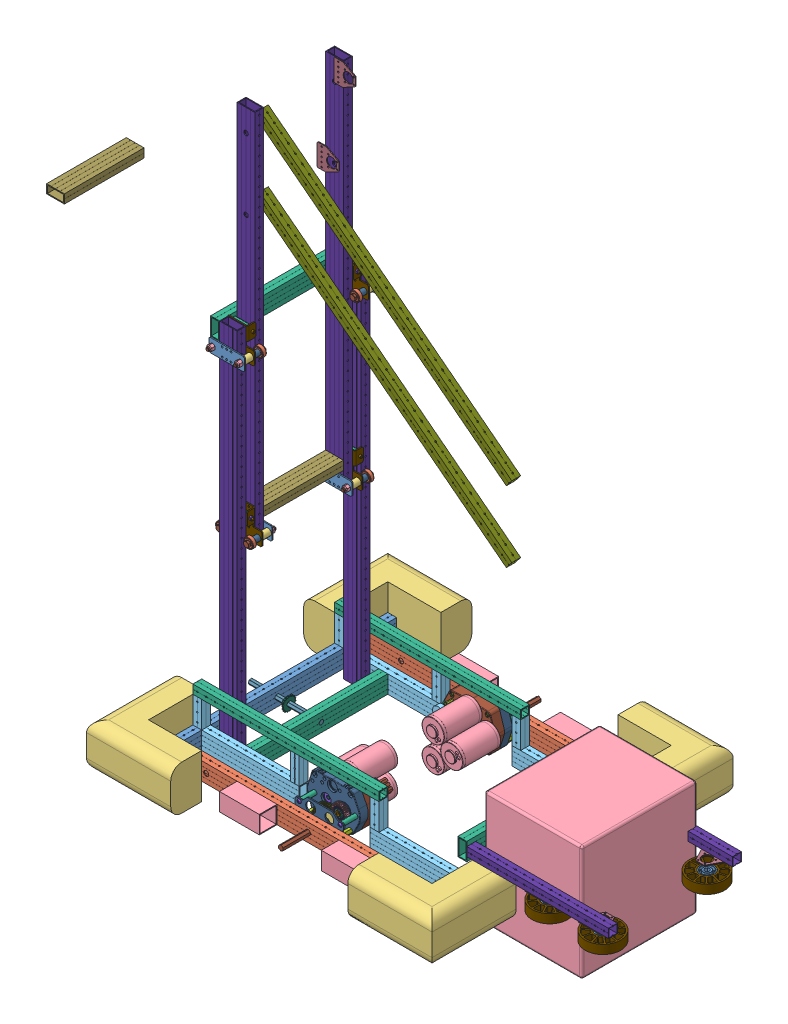
SolidWorks assembly Test Robot 1, configuration Default. Lengths in mm.
Overall size (1417.68 1634.47 868.53).
415 component instances, 100 part files, 60 mates.
Components (placement in the parent):
- Test Base 1-1: Test Base 1 [Default] at (-535.787 40.8668 506.935) size (990.6 169.11 863.6)
  - Base Rear Rail-1: Base Rear Rail [Default] at (282.1219 360.9185 104.1623) size (25.4 50.8 685.8)
  - Base Side Rail-1: Base Side Rail [Default] at (1044.1219 360.9185 789.9623) x (0 0 1) z (-1 0 0) size (25.4 50.8 762)
  - Base Side Rail-2: Base Side Rail [Default] at (1044.1219 360.9185 231.1623) x (0 0 1) z (-1 0 0) size (25.4 50.8 762)
  - Blue Bumper-1: Blue Bumper [Default] at (1171.1219 335.5185 942.3623) x (0 0 -1) z (1 0 0) size (241.3 127 241.3)
  - Blue Bumper-2: Blue Bumper [Default] at (1171.1219 335.5185 78.7623) x (-1 0 0) z (0 0 -1) size (241.3 127 241.3)
  - Bumper Support Bar-2: Bumper Support Bar [Default] at (879.0219 335.5185 166.0294) x (0 0 1) z (-1 0 0) size (50.8 50.8 114.3)
  - Bumper Support Bar-4: Bumper Support Bar [Default] at (586.9219 335.5185 166.0294) x (0 0 1) z (-1 0 0) size (50.8 50.8 114.3)
  - Bumper Support Bar-7: Bumper Support Bar [Default] at (586.9219 335.5185 801.0294) x (0 0 1) z (-1 0 0) size (50.8 50.8 114.3)
  - Bumper Support Bar-8: Bumper Support Bar [Default] at (879.0219 335.5185 801.0294) x (0 0 1) z (-1 0 0) size (50.8 50.8 114.3)
  - Base Side Rail Internal-1: Base Side Rail Internal [Default] at (307.5219 360.9185 307.3623) x (0 0 -1) z (1 0 0) size (25.4 50.8 279.4)
  - Base Side Rail Internal-2: Base Side Rail Internal [Default] at (307.5219 360.9185 713.7623) x (0 0 -1) z (1 0 0) size (25.4 50.8 279.4)
  - Base Side Rail Internal-3: Base Side Rail Internal [Default] at (1044.1219 360.9185 307.3623) x (0 0 1) z (-1 0 0) size (25.4 50.8 279.4)
  - Base Side Rail Internal-4: Base Side Rail Internal [Default] at (1044.1219 360.9185 713.7623) x (0 0 1) z (-1 0 0) size (25.4 50.8 279.4)
  - Frame Crossbar-1: Frame Crossbar [Default] at (1069.5219 360.9185 -48.2377) size (25.4 50.8 381)
  - Base Front Rail-1: Base Front Rail [Default] at (1069.5219 360.9185 104.1623) size (25.4 50.8 152.4)
  - 3 CIM Ball Shifter with WCD Output-1: 3 CIM Ball Shifter with WCD Output [Default] at (711.3612 400.7203 682.3171) x (0 1 0) z (0 0 1) size (169.11 183.68 312.65)
    - 217-2733-001 Rev2-1: 217-2733-001 Rev2 [Default] at (0 53.4162 37.6682) x (0 0 1) z (-0.00054 -1 0) size (7.11 24.61 24.61)
    - 217-2733-001 Rev2-2: 217-2733-001 Rev2 [Default] at (0 53.4162 7.9248) x (0 0 -1) z (-0.038475 0.99926 0) size (7.11 24.61 24.61)
    - 217-2731-001 Rev2-1: 217-2731-001 Rev2 [Default] at (0 0 0.0381) x (-0.099212 0.995066 0) z (0.995066 0.099212 0) size (31.12 7.94 31.12)
    - 217-2789-001 Rev2-1: 217-2789-001 Rev2 [Default] at (0 0 43.2943) x (0 0 -1) z (-0.58471 0.811243 0) size (11.1 38.4 38.4)
    - 217-2778-001 Rev2_NCQ8A075-050M_1-1: 217-2778-001 Rev2_NCQ8A075-050M_1 [Default] at (0 0 -53.848) x (-0.707107 0.707107 0) z (0 0 1) size (31.75 33.34 39.88)
      - 217-2778-002_075A-1: 217-2778-002_075A [Default] at origin size (31.75 33.34 26.92)
      - 217-2778-003_075M-1: 217-2778-003_075M [Default] at (0 0 -8.85) x (0.866025 -0.5 0) z (0 0 1) size (18.95 18.95 35.27)
      - 217-2778-004_075-1: 217-2778-004_075 [Default] at (0 0 10.362) size (21 20.74 0.97)
    - 217-2428-012 Rev2-1: 217-2428-012 Rev2 [Default] at (0 0 -40.386) size (63.5 22.23 2.29)
    - 217-2428-005 Rev1-1: 217-2428-005 Rev1 [Default] at (25.4 0 -19.05) x (-0.557362 -0.83027 0) z (-0.83027 0.557362 0) size (7.33 38.98 6.35)
    - 217-2428-005 Rev1-2: 217-2428-005 Rev1 [Default] at (-25.4 0 -19.05) x (0.667436 0.744667 0) z (0.744667 -0.667436 0) size (7.33 38.98 6.35)
    - SCREW-832-0375-1: SCREW-832-0375 [Default] at (25.4 0 -42.5958) x (0 0 1) z (-0.875404 0.483392 0) size (11.73 7.92 7.92)
    - SCREW-832-0375-2: SCREW-832-0375 [Default] at (-25.4 0 -42.5958) x (0 0 1) z (-0.966319 0.257347 0) size (11.73 7.92 7.92)
    - SCREW-832-0375-3: SCREW-832-0375 [Default] at (25.4 0 5.3848) x (0 0 -1) z (1 0 0) size (11.73 7.92 7.92)
    - SCREW-832-0375-4: SCREW-832-0375 [Default] at (-25.4 0 5.3848) x (0 0 -1) z (0.941463 -0.337115 0) size (11.73 7.92 7.92)
    - SBS1_SBS-0632-0250-1: SBS1_SBS-0632-0250 [Default] at (15.494 0 -36.2458) x (0 0 -1) z (0.854303 -0.519775 0) size (8.57 6.68 6.65)
    - SBS1_SBS-0632-0250-2: SBS1_SBS-0632-0250 [Default] at (-15.494 0 -36.2458) x (0 0 -1) z (0.854303 -0.519775 0) size (8.57 6.68 6.65)
    - 217-4098-100 Rev1-1: 217-4098-100 Rev1 [Default] at (0 0 -16.927) x (-0.503316 0.864103 0) z (0 0 1) size (18.03 19.79 22.46)
      - 217-4098-006 Rev2-1: 217-4098-006 Rev2 [Default] at (0 0 -4.6312) x (0 -1 0) z (0 0 -1) size (18.09 11.02 22.46)
      - 217-4098-006 Rev2-2: 217-4098-006 Rev2 [Default] at (0 0 -4.6312) x (0 1 0) z (0 0 -1) size (18.09 11.02 22.46)
      - 217-3489-001 Rev1-1: 217-3489-001 Rev1 [Default] at (0 0 -4.6312) x (0 0 1) z (-0.980217 -0.197926 0) size (4.77 12.7 12.7)
      - 97633A130_97633A130_grv-1: 97633A130_97633A130_grv [Default] at (0 0 -7.33) x (0 0 -1) z (0.979861 0.199683 0) size (0.64 8.74 7.34)
      - 91251A107_91251A107-1: 91251A107_91251A107 [Default] at (-4.8375 -6.735 -9.4343) x (0 0.863883 -0.503692) z (-1 0 0) size (4.65 4.65 10.79)
      - 91251A107_91251A107-2: 91251A107_91251A107 [Default] at (4.8375 6.735 -9.4343) x (0 0.470889 -0.882193) z (1 0 0) size (4.65 4.65 10.79)
    - 217-2428-017 Rev2-1: 217-2428-017 Rev2 [Default] at (12.7 -21.997 -3.614) x (-0.578458 -0.815712 0) z (0 0 -1) size (14.73 14.73 7.37)
    - 217-2428-016 Rev3_Spur01-1: 217-2428-016 Rev3_Spur01 [Default] at (0 0 -3.614) x (0.873157 -0.48744 0) z (0 0 1) size (40.67 40.74 13.32)
    - 217-2428-019 Rev1-1: 217-2428-019 Rev1 [Default] at (12.7 -21.997 -20.6248) x (0.866025 0.5 0) z (0 0 1) size (50.8 19.05 1.57)
    - 217-2428-006 Rev1-1: 217-2428-006 Rev1 [Default] at (32.079 -14.2875 -9.525) x (-0.752416 0.658689 0) z (0.658689 0.752416 0) size (7.33 19.93 6.35)
    - 217-2428-006 Rev1-2: 217-2428-006 Rev1 [Default] at (-3.6662 -34.925 -9.525) x (0.84498 0.534798 0) z (0.534798 -0.84498 0) size (7.33 19.93 6.35)
    - SCREW-832-0375-5: SCREW-832-0375 [Default] at (32.079 -14.2875 4.7498) x (0 0 -1) z (0.980613 0.195955 0) size (11.73 7.92 7.92)
    - SCREW-832-0375-6: SCREW-832-0375 [Default] at (-3.6662 -34.925 5.3848) x (0 0 -1) z (-0.672515 -0.740083 0) size (11.73 7.92 7.92)
    - SCREW-832-0375-7: SCREW-832-0375 [Default] at (-3.6662 -34.925 -22.8346) x (0 0 1) z (0.948865 0.315681 0) size (11.73 7.92 7.92)
    - SCREW-832-0375-8: SCREW-832-0375 [Default] at (32.079 -14.2875 -22.8346) x (0 0 1) z (-0.875404 0.483392 0) size (11.73 7.92 7.92)
    - 217-2614-001_12t-1: 217-2614-001_12t [Default] at (36.9798 39.6868 15.8623) x (-0.087156 0.996195 0) z (0 0 1) size (18.29 18.29 19)
    - 217-2761-001 rev1-1: 217-2761-001 rev1 [Default] at (33.1943 39.3556 16.1) x (0.087156 -0.996195 0) z (0 0 1) size (2 2 20)
    - 217-2761-001 rev1-2: 217-2761-001 rev1 [Default] at (-40.7653 40.018 16.1) x (0.087156 0.996195 0) z (0 0 1) size (2 2 20)
    - 217-2614-001_12t-2: 217-2614-001_12t [Default] at (-36.9798 39.6868 15.8623) x (0.087156 0.996195 0) z (0 0 1) size (18.29 18.29 19)
    - 217-2614-001_12t-3: 217-2614-001_12t [Default] at (0 92.8624 15.8623) x (0.97459 0.223996 0) z (0 0 1) size (18.29 18.29 19)
    - 217-2761-001 rev1-3: 217-2761-001 rev1 [Default] at (-0.8512 96.5658 16.1) x (0.97459 0.223996 0) z (0 0 1) size (2 2 20)
    - 217-3195-002 rev2-1: 217-3195-002 rev2 [Default] at (0 0 50.546) x (-1 0 0) z (0 0 -1) size (114.31 152.24 24.96)
    - 217-3195-001 Rev1-1: 217-3195-001 Rev1 [Default] at origin size (113.41 152.24 26.86)
    - Nylock Nut_NNY2520-ZC-1: Nylock Nut_NNY2520-ZC [Default] at (48.8823 73.025 37.846) x (0 0.866025 -0.5) z (-1 0 0) size (12.85 11.89 7.62)
    - Nylock Nut_NNY2520-ZC-2: Nylock Nut_NNY2520-ZC [Default] at (48.8823 -3.175 37.846) x (0 0 -1) z (-1 0 0) size (12.85 11.89 7.62)
    - Nylock Nut_NNY2520-ZC-3: Nylock Nut_NNY2520-ZC [Default] at (44.45 85.725 7.8613) x (0 1 0) z (0 0 -1) size (12.85 11.89 7.62)
    - 276-1027-001-1: 276-1027-001 [Default] at (47.625 58.1787 6.35) x (0 1 0) z (-1 0 0) size (8.61 5.64 9.94)
    - 276-1027-001-2: 276-1027-001 [Default] at (-47.625 58.1787 6.35) x (0 -1 0) z (1 0 0) size (8.61 5.64 9.94)
    - SCREW-832-1750-1: SCREW-832-1750 [Default] at (-47.625 58.1787 47.0408) x (0 0 -1) z (-0.960822 -0.277167 0) size (46.66 7.92 7.92)
    - SCREW-832-1750-2: SCREW-832-1750 [Default] at (47.625 58.1787 47.0408) x (0 0 -1) z (-0.960822 -0.277167 0) size (46.66 7.92 7.92)
    - Nylock Nut_NNY2520-ZC-4: Nylock Nut_NNY2520-ZC [Default] at (44.45 -15.875 7.8613) x (0 1 0) z (0 0 -1) size (12.85 11.89 7.62)
    - 217-2428-004 Rev3-1: 217-2428-004 Rev3 [Default] at (0 53.4162 22.7711) x (-0.709585 0.70462 0) z (0 0 1) size (11 9.53 43.92)
    - SBS1_SBS-2520-1625SS-1: SBS1_SBS-2520-1625SS [Default] at (44.45 85.725 42.4688) x (0 0 -1) z (-0.251219 0.96793 0) size (45.3 11.2 11.18)
    - SBS1_SBS-2520-1625SS-2: SBS1_SBS-2520-1625SS [Default] at (44.45 -15.875 42.4688) x (0 0 -1) z (-0.251219 0.96793 0) size (45.3 11.2 11.18)
    - SBS1_SBS2520-1750-1: SBS1_SBS2520-1750 [Default] at (-44.45 85.725 7.4422) x (0 0 1) z (-0.031478 0.999504 0) size (48.48 11.22 11.17)
    - SBS1_SBS2520-1750-2: SBS1_SBS2520-1750 [Default] at (-44.45 -15.875 7.4422) x (0 0 1) z (-0.937114 -0.349025 0) size (48.48 11.22 11.17)
    - 217-2428-021 Rev1-1: 217-2428-021 Rev1 [Default] at (0 53.4162 9.5123) x (0.451333 -0.892356 0) z (0 0 1) size (15.88 15.88 3.17)
    - 217-2428-029 Rev1-1: 217-2428-029 Rev1 [Default] at (0 53.4162 36.957) x (0.999846 0.017557 0) z (0 0 1) size (15.88 15.88 1.12)
    - Grayhill Lock Washer-1: Grayhill Lock Washer [Default] at (12.7 -21.997 -18.6817) x (0.467173 -0.884166 0) z (0 0 1) size (19.69 19.69 0.74)
    - Grayhill Nut-1: Grayhill Nut [Default] at (12.7 -21.997 -17.0434) x (0.984088 0.177684 0) z (0 0 1) size (18.33 15.88 2.54)
    - 217-2000-1: 217-2000 [Default] at (0 92.8624 0) x (0 0 -1) z (0.223996 -0.97459 0) size (150.2 64.01 64.01)
    - 217-2000-2: 217-2000 [Default] at (-36.9798 39.6868 0) x (0 0 -1) z (0.996195 -0.087156 0) size (150.2 64.01 64.01)
    - 217-2000-3: 217-2000 [Default] at (36.9798 39.6868 0) x (0 0 -1) z (0.996195 0.087156 0) size (150.2 64.01 64.01)
    - Grahill Encoder-1: Grahill Encoder [Default] at (12.7 -21.997 -16.1798) x (-0.580071 0.814566 0) z (-0.814566 -0.580071 0) size (31.75 31.12 31.75)
    - 217-3195-009 Rev1_wcd 2-1: 217-3195-009 Rev1_wcd 2 [Default] at (0 85.725 50.546) x (-0.998427 -0.056065 0) z (0 0 1) size (12.7 12.7 41.27)
    - 217-3195-006 Rev1_WCD-1: 217-3195-006 Rev1_WCD [Default] at (-44.45 85.725 44.1452) x (0.5 0.866025 0) z (0 0 1) size (12.7 14.66 47.62)
    - 217-3195-009 Rev1_wcd 2-2: 217-3195-009 Rev1_wcd 2 [Default] at (0 -31.75 50.546) x (0.947633 0.319361 0) z (0 0 1) size (12.7 12.7 41.27)
    - 217-3195-006 Rev1_WCD-2: 217-3195-006 Rev1_WCD [Default] at (-44.45 -15.875 44.1452) x (0.5 -0.866025 0) z (0 0 1) size (12.7 14.66 47.62)
    - Nylock Nut_NNY2520-ZC-5: Nylock Nut_NNY2520-ZC [Default] at (0 -31.75 45.0723) x (-0.5 0.866025 0) z (0 0 -1) size (12.85 11.89 7.62)
    - Nylock Nut_NNY2520-ZC-6: Nylock Nut_NNY2520-ZC [Default] at (0 85.725 45.0723) x (-0.5 0.866025 0) z (0 0 -1) size (12.85 11.89 7.62)
    - SBS1_SBS-2520-2250-1: SBS1_SBS-2520-2250 [Default] at (0 -31.75 98.298) x (0 0 -1) z (-0.933488 -0.358607 0) size (61.18 11.22 11.17)
    - SBS1_SBS2520-0625ZC-1: SBS1_SBS2520-0625ZC [Default] at (-44.45 85.725 98.298) x (0 0 -1) z (0.400817 0.916158 0) size (19.57 11.22 11.17)
    - SBS1_SBS2520-0625ZC-2: SBS1_SBS2520-0625ZC [Default] at (-44.45 -15.875 98.298) x (0 0 -1) z (-0.75178 -0.659414 0) size (19.57 11.22 11.17)
    - SBS1_SBS-2520-2250-2: SBS1_SBS-2520-2250 [Default] at (0 85.725 98.298) x (0 0 -1) z (0.056677 -0.998393 0) size (61.18 11.22 11.17)
    - 217-3195-003 rev2-1: 217-3195-003 rev2 [Default] at (0 0 94.9452) size (88.62 139.7 3.17)
    - 217-2617-003 Rev1-1: 217-2617-003 Rev1 [Default] at (-39.878 35.5392 121.8535) x (-0.5 -0.866025 0) z (0 0 1) size (14.66 12.7 152.4)
    - 217-3109-001 Rev1-1: 217-3109-001 Rev1 [Default] at (-39.878 35.5392 49.1808) x (0 0 1) z (0.312889 -0.94979 0) size (7.94 28.57 28.57)
    - 217-2734-001 Rev3-1: 217-2734-001 Rev3 [Default] at (-39.878 35.5392 98.1202) x (1 0 0) z (0 1 0) size (31.12 7.94 31.12)
    - 217-2617-004 Rev1_97431A340_grv-1: 217-2617-004 Rev1_97431A340_grv [Default] at (-39.878 35.5392 54.8961) x (0 0 1) z (-0.124043 -0.992277 0) size (1.07 20.42 18.58)
    - 217-2617-004 Rev1_97431A340_grv-2: 217-2617-004 Rev1_97431A340_grv [Default] at (0 0 69.215) x (0 0 1) z (-0.124043 -0.992277 0) size (1.07 20.42 18.58)
    - 217-2702-001_20t-1: 217-2702-001_20t [Default] at (0 0 62.357) x (0.998435 0.055929 0) z (0 0 1) size (28.2 28.2 12.65)
    - 217-2715-002 Rev1_64t-1: 217-2715-002 Rev1_64t [Default] at (-39.878 35.5392 61.7541) x (0.866025 -0.5 0) z (0 0 1) size (84.3 84.3 12.65)
    - 217-2704-001_24-1: 217-2704-001_24 [Default] at (0 0 62.357) x (0.450781 0.892635 0) z (0 0 -1) size (33.29 33.29 12.65)
    - 217-2714-002 Rev1_60t-1: 217-2714-002 Rev1_60t [Default] at (-39.878 35.5392 61.7541) x (0.866025 -0.5 0) z (0 0 1) size (78.95 78.95 12.65)
    - 217-3221-002 Rev1-1: 217-3221-002 Rev1 [Default] at (-39.878 35.5392 61.7414) x (0 -1 0) z (0 0 1) size (71.39 71.45 12.62)
    - 217-2705-001_30t-1: 217-2705-001_30t [Default] at (0 0 62.357) x (0.547654 -0.836705 0) z (0 0 1) size (41.01 41.12 12.65)
    - 217-2712-002 Rev1_50t-1: 217-2712-002 Rev1_50t [Default] at (-39.878 35.5392 61.7541) x (0.866025 -0.5 0) z (0 0 1) size (66.7 66.76 12.65)
    - 217-2706-001_34t-1: 217-2706-001_34t [Default] at (0 0 62.357) x (0.998435 0.055929 0) z (0 0 1) size (46.46 46.56 12.65)
    - 217-3288-001 Rev3-1: 217-3288-001 Rev3 [Default] at (0 0 0.0889) x (0.055929 -0.998435 0) z (0 0 1) size (99.51 99.53 98.3)
      - 217-2428-008 Rev2-1: 217-2428-008 Rev2 [Default] at (0 0 10.2679) size (31.75 31.75 1.59)
      - 217-2428-028 Rev1_97633A250-1: 217-2428-028 Rev1_97633A250 [Default] at (0 0 37.1221) x (0 0 1) z (0.9357 -0.352797 0) size (1.07 23.39 21.18)
      - 217-4099-000 Rev2_high gear-1: 217-4099-000 Rev2_high gear [Default] x (-1 0 0) z (0 0 1) size (22.23 22.23 98.3)
        - 217-4098-005 Rev1_91612A226-1: 217-4098-005 Rev1_91612A226 [Default] at (0 0 46.2661) x (-0.144757 0 0.989467) z (0 -1 0) size (3.02 3.15 18.22)
        - 217-4098-003 Rev2-1: 217-4098-003 Rev2 [Default] x (1 0 0) z (0 0 -1) size (22.23 22.23 55.94)
        - 217-4099-002 Rev3-1: 217-4099-002 Rev3 [Default] at (0 0 53.467) x (0 0 1) z (-1 0 0) size (40.96 12.73 14.67)
        - 217-4098-004 Rev1-1: 217-4098-004 Rev1 [Default] at (0 0 14.2494) x (0.393904 0.919152 0) z (0 0 1) size (11.68 11.68 56)
      - 217-2428-007 Rev1-1: 217-2428-007 Rev1 [Default] at (7.809 4.5085 14.2494) x (-0.69071 0.455693 -0.561483) z (-0.67559 -0.683536 0.276329) size (6.35 6.35 6.35)
      - 217-2428-007 Rev1-2: 217-2428-007 Rev1 [Default] at (5.4343 3.1375 26.9494) x (-0.162331 -0.978398 0.128005) z (0.857281 -0.204076 -0.472676) size (6.35 6.35 6.35)
      - 217-3212-101 Rev1-1: 217-3212-101 Rev1 [Default] at (-11.5751 10.4131 45.3224) x (0.923728 0.383049 0) z (0 0 -1) size (46.46 46.56 12.7)
        - 217-2428-022 Rev1-1: 217-2428-022 Rev1 [Default] at (6.7035 14.0527 24.6087) size (28.57 28.57 6.1)
        - 217-3212-001 Rev1_34t-1: 217-3212-001 Rev1_34t [Default] at (6.7035 14.0527 27.9107) size (46.46 46.56 11.11)
      - 217-3222-101 Rev1-1: 217-3222-101 Rev1 [Default] at (21.0941 -5.2804 52.7371) x (-0.889163 -0.457591 0) z (0 0 -1) size (73.87 73.92 12.7)
        - 217-2428-022 Rev1-1: 217-2428-022 Rev1 [Default] at (16.3398 14.3476 19.3234) size (28.57 28.57 6.1)
        - 217-3222-001 Rev1_Spur01-1: 217-3222-001 Rev1_Spur01 [Default] at (16.3398 14.3476 22.6254) x (0.999377 0.0353 0) z (0 0 1) size (71.39 71.45 11.11)
      - 217-2428-007 Rev1-3: 217-2428-007 Rev1 [Default] at (-5.4343 3.1375 26.9494) x (0.928483 0.348617 0.128005) z (-0.251905 0.844465 -0.472676) size (6.35 6.35 6.35)
      - 217-2428-007 Rev1-4: 217-2428-007 Rev1 [Default] at (0 -6.275 26.9494) x (-0.766153 0.629782 0.128005) z (-0.605376 -0.640389 -0.472676) size (6.35 6.35 6.35)
      - 217-2428-007 Rev1-5: 217-2428-007 Rev1 [Default] at (-7.809 4.5085 14.2494) x (-0.049287 -0.826019 -0.561483) z (0.929754 -0.24331 0.276329) size (6.35 6.35 6.35)
      - 217-2428-007 Rev1-6: 217-2428-007 Rev1 [Default] at (0 -9.017 14.2494) x (0.739997 0.370326 -0.561483) z (-0.254164 0.926846 0.276329) size (6.35 6.35 6.35)
    - 217-3210-001 Rev1_30t-1: 217-3210-001 Rev1_30t [Default] at (0 53.4162 30.0736) x (-0.966828 0.255427 0) z (0 0 1) size (41.01 41.12 12.65)
    - 217-2711-002 Rev1_50t-1: 217-2711-002 Rev1_50t [Default] at (0 53.4162 17.4244) x (0.262208 -0.965011 0) z (0 0 1) size (66.7 66.76 12.65)
  - 3 CIM Ball Shifter with WCD Output-2: 3 CIM Ball Shifter with WCD Output [Default] at (640.2827 400.7203 338.8075) x (0 1 0) z (0 0 -1) size (169.11 183.68 312.65)
    - 217-2733-001 Rev2-1: 217-2733-001 Rev2 [Default] at (0 53.4162 37.6682) x (0 0 1) z (-0.00054 -1 0) size (7.11 24.61 24.61)
    - 217-2733-001 Rev2-2: 217-2733-001 Rev2 [Default] at (0 53.4162 7.9248) x (0 0 -1) z (-0.038475 0.99926 0) size (7.11 24.61 24.61)
    - 217-2731-001 Rev2-1: 217-2731-001 Rev2 [Default] at (0 0 0.0381) x (-0.099212 0.995066 0) z (0.995066 0.099212 0) size (31.12 7.94 31.12)
    - 217-2789-001 Rev2-1: 217-2789-001 Rev2 [Default] at (0 0 43.2943) x (0 0 -1) z (-0.58471 0.811243 0) size (11.1 38.4 38.4)
    - 217-2778-001 Rev2_NCQ8A075-050M_1-1: 217-2778-001 Rev2_NCQ8A075-050M_1 [Default] at (0 0 -53.848) x (-0.707107 0.707107 0) z (0 0 1) size (31.75 33.34 39.88)
      - 217-2778-002_075A-1: 217-2778-002_075A [Default] at origin size (31.75 33.34 26.92)
      - 217-2778-003_075M-1: 217-2778-003_075M [Default] at (0 0 -8.85) x (0.866025 -0.5 0) z (0 0 1) size (18.95 18.95 35.27)
      - 217-2778-004_075-1: 217-2778-004_075 [Default] at (0 0 10.362) size (21 20.74 0.97)
    - 217-2428-012 Rev2-1: 217-2428-012 Rev2 [Default] at (0 0 -40.386) size (63.5 22.23 2.29)
    - 217-2428-005 Rev1-1: 217-2428-005 Rev1 [Default] at (25.4 0 -19.05) x (-0.557362 -0.83027 0) z (-0.83027 0.557362 0) size (7.33 38.98 6.35)
    - 217-2428-005 Rev1-2: 217-2428-005 Rev1 [Default] at (-25.4 0 -19.05) x (0.667436 0.744667 0) z (0.744667 -0.667436 0) size (7.33 38.98 6.35)
    - SCREW-832-0375-1: SCREW-832-0375 [Default] at (25.4 0 -42.5958) x (0 0 1) z (-0.875404 0.483392 0) size (11.73 7.92 7.92)
    - SCREW-832-0375-2: SCREW-832-0375 [Default] at (-25.4 0 -42.5958) x (0 0 1) z (-0.966319 0.257347 0) size (11.73 7.92 7.92)
    - SCREW-832-0375-3: SCREW-832-0375 [Default] at (25.4 0 5.3848) x (0 0 -1) z (1 0 0) size (11.73 7.92 7.92)
    - SCREW-832-0375-4: SCREW-832-0375 [Default] at (-25.4 0 5.3848) x (0 0 -1) z (0.941463 -0.337115 0) size (11.73 7.92 7.92)
    - SBS1_SBS-0632-0250-1: SBS1_SBS-0632-0250 [Default] at (15.494 0 -36.2458) x (0 0 -1) z (0.854303 -0.519775 0) size (8.57 6.68 6.65)
    - SBS1_SBS-0632-0250-2: SBS1_SBS-0632-0250 [Default] at (-15.494 0 -36.2458) x (0 0 -1) z (0.854303 -0.519775 0) size (8.57 6.68 6.65)
    - 217-4098-100 Rev1-1: 217-4098-100 Rev1 [Default] at (0 0 -16.927) x (-0.503316 0.864103 0) z (0 0 1) size (18.03 19.79 22.46)
      - 217-4098-006 Rev2-1: 217-4098-006 Rev2 [Default] at (0 0 -4.6312) x (0 -1 0) z (0 0 -1) size (18.09 11.02 22.46)
      - 217-4098-006 Rev2-2: 217-4098-006 Rev2 [Default] at (0 0 -4.6312) x (0 1 0) z (0 0 -1) size (18.09 11.02 22.46)
      - 217-3489-001 Rev1-1: 217-3489-001 Rev1 [Default] at (0 0 -4.6312) x (0 0 1) z (-0.980217 -0.197926 0) size (4.77 12.7 12.7)
      - 97633A130_97633A130_grv-1: 97633A130_97633A130_grv [Default] at (0 0 -7.33) x (0 0 -1) z (0.979861 0.199683 0) size (0.64 8.74 7.34)
      - 91251A107_91251A107-1: 91251A107_91251A107 [Default] at (-4.8375 -6.735 -9.4343) x (0 0.863883 -0.503692) z (-1 0 0) size (4.65 4.65 10.79)
      - 91251A107_91251A107-2: 91251A107_91251A107 [Default] at (4.8375 6.735 -9.4343) x (0 0.470889 -0.882193) z (1 0 0) size (4.65 4.65 10.79)
    - 217-2428-017 Rev2-1: 217-2428-017 Rev2 [Default] at (12.7 -21.997 -3.614) x (-0.578458 -0.815712 0) z (0 0 -1) size (14.73 14.73 7.37)
    - 217-2428-016 Rev3_Spur01-1: 217-2428-016 Rev3_Spur01 [Default] at (0 0 -3.614) x (0.873157 -0.48744 0) z (0 0 1) size (40.67 40.74 13.32)
    - 217-2428-019 Rev1-1: 217-2428-019 Rev1 [Default] at (12.7 -21.997 -20.6248) x (0.866025 0.5 0) z (0 0 1) size (50.8 19.05 1.57)
    - 217-2428-006 Rev1-1: 217-2428-006 Rev1 [Default] at (32.079 -14.2875 -9.525) x (-0.752416 0.658689 0) z (0.658689 0.752416 0) size (7.33 19.93 6.35)
    - 217-2428-006 Rev1-2: 217-2428-006 Rev1 [Default] at (-3.6662 -34.925 -9.525) x (0.84498 0.534798 0) z (0.534798 -0.84498 0) size (7.33 19.93 6.35)
    - SCREW-832-0375-5: SCREW-832-0375 [Default] at (32.079 -14.2875 4.7498) x (0 0 -1) z (0.980613 0.195955 0) size (11.73 7.92 7.92)
    - SCREW-832-0375-6: SCREW-832-0375 [Default] at (-3.6662 -34.925 5.3848) x (0 0 -1) z (-0.672515 -0.740083 0) size (11.73 7.92 7.92)
    - SCREW-832-0375-7: SCREW-832-0375 [Default] at (-3.6662 -34.925 -22.8346) x (0 0 1) z (0.948865 0.315681 0) size (11.73 7.92 7.92)
    - SCREW-832-0375-8: SCREW-832-0375 [Default] at (32.079 -14.2875 -22.8346) x (0 0 1) z (-0.875404 0.483392 0) size (11.73 7.92 7.92)
    - 217-2614-001_12t-1: 217-2614-001_12t [Default] at (36.9798 39.6868 15.8623) x (-0.087156 0.996195 0) z (0 0 1) size (18.29 18.29 19)
    - 217-2761-001 rev1-1: 217-2761-001 rev1 [Default] at (33.1943 39.3556 16.1) x (0.087156 -0.996195 0) z (0 0 1) size (2 2 20)
    - 217-2761-001 rev1-2: 217-2761-001 rev1 [Default] at (-40.7653 40.018 16.1) x (0.087156 0.996195 0) z (0 0 1) size (2 2 20)
    - 217-2614-001_12t-2: 217-2614-001_12t [Default] at (-36.9798 39.6868 15.8623) x (0.087156 0.996195 0) z (0 0 1) size (18.29 18.29 19)
    - 217-2614-001_12t-3: 217-2614-001_12t [Default] at (0 92.8624 15.8623) x (0.97459 0.223996 0) z (0 0 1) size (18.29 18.29 19)
    - 217-2761-001 rev1-3: 217-2761-001 rev1 [Default] at (-0.8512 96.5658 16.1) x (0.97459 0.223996 0) z (0 0 1) size (2 2 20)
    - 217-3195-002 rev2-1: 217-3195-002 rev2 [Default] at (0 0 50.546) x (-1 0 0) z (0 0 -1) size (114.31 152.24 24.96)
    - 217-3195-001 Rev1-1: 217-3195-001 Rev1 [Default] at origin size (113.41 152.24 26.86)
    - Nylock Nut_NNY2520-ZC-1: Nylock Nut_NNY2520-ZC [Default] at (48.8823 73.025 37.846) x (0 0.866025 -0.5) z (-1 0 0) size (12.85 11.89 7.62)
    - Nylock Nut_NNY2520-ZC-2: Nylock Nut_NNY2520-ZC [Default] at (48.8823 -3.175 37.846) x (0 0 -1) z (-1 0 0) size (12.85 11.89 7.62)
    - Nylock Nut_NNY2520-ZC-3: Nylock Nut_NNY2520-ZC [Default] at (44.45 85.725 7.8613) x (0 1 0) z (0 0 -1) size (12.85 11.89 7.62)
    - 276-1027-001-1: 276-1027-001 [Default] at (47.625 58.1787 6.35) x (0 1 0) z (-1 0 0) size (8.61 5.64 9.94)
    - 276-1027-001-2: 276-1027-001 [Default] at (-47.625 58.1787 6.35) x (0 -1 0) z (1 0 0) size (8.61 5.64 9.94)
    - SCREW-832-1750-1: SCREW-832-1750 [Default] at (-47.625 58.1787 47.0408) x (0 0 -1) z (-0.960822 -0.277167 0) size (46.66 7.92 7.92)
    - SCREW-832-1750-2: SCREW-832-1750 [Default] at (47.625 58.1787 47.0408) x (0 0 -1) z (-0.960822 -0.277167 0) size (46.66 7.92 7.92)
    - Nylock Nut_NNY2520-ZC-4: Nylock Nut_NNY2520-ZC [Default] at (44.45 -15.875 7.8613) x (0 1 0) z (0 0 -1) size (12.85 11.89 7.62)
    - 217-2428-004 Rev3-1: 217-2428-004 Rev3 [Default] at (0 53.4162 22.7711) x (-0.709585 0.70462 0) z (0 0 1) size (11 9.53 43.92)
    - SBS1_SBS-2520-1625SS-1: SBS1_SBS-2520-1625SS [Default] at (44.45 85.725 42.4688) x (0 0 -1) z (-0.251219 0.96793 0) size (45.3 11.2 11.18)
    - SBS1_SBS-2520-1625SS-2: SBS1_SBS-2520-1625SS [Default] at (44.45 -15.875 42.4688) x (0 0 -1) z (-0.251219 0.96793 0) size (45.3 11.2 11.18)
    - SBS1_SBS2520-1750-1: SBS1_SBS2520-1750 [Default] at (-44.45 85.725 7.4422) x (0 0 1) z (-0.031478 0.999504 0) size (48.48 11.22 11.17)
    - SBS1_SBS2520-1750-2: SBS1_SBS2520-1750 [Default] at (-44.45 -15.875 7.4422) x (0 0 1) z (-0.937114 -0.349025 0) size (48.48 11.22 11.17)
    - 217-2428-021 Rev1-1: 217-2428-021 Rev1 [Default] at (0 53.4162 9.5123) x (0.451333 -0.892356 0) z (0 0 1) size (15.88 15.88 3.17)
    - 217-2428-029 Rev1-1: 217-2428-029 Rev1 [Default] at (0 53.4162 36.957) x (0.999846 0.017557 0) z (0 0 1) size (15.88 15.88 1.12)
    - Grayhill Lock Washer-1: Grayhill Lock Washer [Default] at (12.7 -21.997 -18.6817) x (0.467173 -0.884166 0) z (0 0 1) size (19.69 19.69 0.74)
    - Grayhill Nut-1: Grayhill Nut [Default] at (12.7 -21.997 -17.0434) x (0.984088 0.177684 0) z (0 0 1) size (18.33 15.88 2.54)
    - 217-2000-1: 217-2000 [Default] at (0 92.8624 0) x (0 0 -1) z (0.223996 -0.97459 0) size (150.2 64.01 64.01)
    - 217-2000-2: 217-2000 [Default] at (-36.9798 39.6868 0) x (0 0 -1) z (0.996195 -0.087156 0) size (150.2 64.01 64.01)
    - 217-2000-3: 217-2000 [Default] at (36.9798 39.6868 0) x (0 0 -1) z (0.996195 0.087156 0) size (150.2 64.01 64.01)
    - Grahill Encoder-1: Grahill Encoder [Default] at (12.7 -21.997 -16.1798) x (-0.580071 0.814566 0) z (-0.814566 -0.580071 0) size (31.75 31.12 31.75)
    - 217-3195-009 Rev1_wcd 2-1: 217-3195-009 Rev1_wcd 2 [Default] at (0 85.725 50.546) x (-0.998427 -0.056065 0) z (0 0 1) size (12.7 12.7 41.27)
    - 217-3195-006 Rev1_WCD-1: 217-3195-006 Rev1_WCD [Default] at (-44.45 85.725 44.1452) x (0.5 0.866025 0) z (0 0 1) size (12.7 14.66 47.62)
    - 217-3195-009 Rev1_wcd 2-2: 217-3195-009 Rev1_wcd 2 [Default] at (0 -31.75 50.546) x (0.947633 0.319361 0) z (0 0 1) size (12.7 12.7 41.27)
    - 217-3195-006 Rev1_WCD-2: 217-3195-006 Rev1_WCD [Default] at (-44.45 -15.875 44.1452) x (0.5 -0.866025 0) z (0 0 1) size (12.7 14.66 47.62)
    - Nylock Nut_NNY2520-ZC-5: Nylock Nut_NNY2520-ZC [Default] at (0 -31.75 45.0723) x (-0.5 0.866025 0) z (0 0 -1) size (12.85 11.89 7.62)
    - Nylock Nut_NNY2520-ZC-6: Nylock Nut_NNY2520-ZC [Default] at (0 85.725 45.0723) x (-0.5 0.866025 0) z (0 0 -1) size (12.85 11.89 7.62)
    - SBS1_SBS-2520-2250-1: SBS1_SBS-2520-2250 [Default] at (0 -31.75 98.298) x (0 0 -1) z (-0.933488 -0.358607 0) size (61.18 11.22 11.17)
    - SBS1_SBS2520-0625ZC-1: SBS1_SBS2520-0625ZC [Default] at (-44.45 85.725 98.298) x (0 0 -1) z (0.400817 0.916158 0) size (19.57 11.22 11.17)
    - SBS1_SBS2520-0625ZC-2: SBS1_SBS2520-0625ZC [Default] at (-44.45 -15.875 98.298) x (0 0 -1) z (-0.75178 -0.659414 0) size (19.57 11.22 11.17)
    - SBS1_SBS-2520-2250-2: SBS1_SBS-2520-2250 [Default] at (0 85.725 98.298) x (0 0 -1) z (0.056677 -0.998393 0) size (61.18 11.22 11.17)
    - 217-3195-003 rev2-1: 217-3195-003 rev2 [Default] at (0 0 94.9452) size (88.62 139.7 3.17)
    - 217-2617-003 Rev1-1: 217-2617-003 Rev1 [Default] at (-39.878 35.5392 121.8535) x (-0.5 -0.866025 0) z (0 0 1) size (14.66 12.7 152.4)
    - 217-3109-001 Rev1-1: 217-3109-001 Rev1 [Default] at (-39.878 35.5392 49.1808) x (0 0 1) z (0.312889 -0.94979 0) size (7.94 28.57 28.57)
    - 217-2734-001 Rev3-1: 217-2734-001 Rev3 [Default] at (-39.878 35.5392 98.1202) x (1 0 0) z (0 1 0) size (31.12 7.94 31.12)
    - 217-2617-004 Rev1_97431A340_grv-1: 217-2617-004 Rev1_97431A340_grv [Default] at (-39.878 35.5392 54.8961) x (0 0 1) z (-0.124043 -0.992277 0) size (1.07 20.42 18.58)
    - 217-2617-004 Rev1_97431A340_grv-2: 217-2617-004 Rev1_97431A340_grv [Default] at (0 0 69.215) x (0 0 1) z (-0.124043 -0.992277 0) size (1.07 20.42 18.58)
    - 217-2702-001_20t-1: 217-2702-001_20t [Default] at (0 0 62.357) x (0.998435 0.055929 0) z (0 0 1) size (28.2 28.2 12.65)
    - 217-2715-002 Rev1_64t-1: 217-2715-002 Rev1_64t [Default] at (-39.878 35.5392 61.7541) x (0.866025 -0.5 0) z (0 0 1) size (84.3 84.3 12.65)
    - 217-2704-001_24-1: 217-2704-001_24 [Default] at (0 0 62.357) x (0.450781 0.892635 0) z (0 0 -1) size (33.29 33.29 12.65)
    - 217-2714-002 Rev1_60t-1: 217-2714-002 Rev1_60t [Default] at (-39.878 35.5392 61.7541) x (0.866025 -0.5 0) z (0 0 1) size (78.95 78.95 12.65)
    - 217-3221-002 Rev1-1: 217-3221-002 Rev1 [Default] at (-39.878 35.5392 61.7414) x (0 -1 0) z (0 0 1) size (71.39 71.45 12.62)
    - 217-2705-001_30t-1: 217-2705-001_30t [Default] at (0 0 62.357) x (0.547654 -0.836705 0) z (0 0 1) size (41.01 41.12 12.65)
    - 217-2712-002 Rev1_50t-1: 217-2712-002 Rev1_50t [Default] at (-39.878 35.5392 61.7541) x (0.866025 -0.5 0) z (0 0 1) size (66.7 66.76 12.65)
    - 217-2706-001_34t-1: 217-2706-001_34t [Default] at (0 0 62.357) x (0.998435 0.055929 0) z (0 0 1) size (46.46 46.56 12.65)
    - 217-3288-001 Rev3-1: 217-3288-001 Rev3 [Default] at (0 0 0.0889) x (0.055929 -0.998435 0) z (0 0 1) size (99.51 99.53 98.3)
      - 217-2428-008 Rev2-1: 217-2428-008 Rev2 [Default] at (0 0 10.2679) size (31.75 31.75 1.59)
      - 217-2428-028 Rev1_97633A250-1: 217-2428-028 Rev1_97633A250 [Default] at (0 0 37.1221) x (0 0 1) z (0.9357 -0.352797 0) size (1.07 23.39 21.18)
      - 217-4099-000 Rev2_high gear-1: 217-4099-000 Rev2_high gear [Default] x (-1 0 0) z (0 0 1) size (22.23 22.23 98.3)
        - 217-4098-005 Rev1_91612A226-1: 217-4098-005 Rev1_91612A226 [Default] at (0 0 46.2661) x (-0.144757 0 0.989467) z (0 -1 0) size (3.02 3.15 18.22)
        - 217-4098-003 Rev2-1: 217-4098-003 Rev2 [Default] x (1 0 0) z (0 0 -1) size (22.23 22.23 55.94)
        - 217-4099-002 Rev3-1: 217-4099-002 Rev3 [Default] at (0 0 53.467) x (0 0 1) z (-1 0 0) size (40.96 12.73 14.67)
        - 217-4098-004 Rev1-1: 217-4098-004 Rev1 [Default] at (0 0 14.2494) x (0.393904 0.919152 0) z (0 0 1) size (11.68 11.68 56)
      - 217-2428-007 Rev1-1: 217-2428-007 Rev1 [Default] at (7.809 4.5085 14.2494) x (-0.69071 0.455693 -0.561483) z (-0.67559 -0.683536 0.276329) size (6.35 6.35 6.35)
      - 217-2428-007 Rev1-2: 217-2428-007 Rev1 [Default] at (5.4343 3.1375 26.9494) x (-0.162331 -0.978398 0.128005) z (0.857281 -0.204076 -0.472676) size (6.35 6.35 6.35)
      - 217-3212-101 Rev1-1: 217-3212-101 Rev1 [Default] at (-11.5751 10.4131 45.3224) x (0.923728 0.383049 0) z (0 0 -1) size (46.46 46.56 12.7)
        - 217-2428-022 Rev1-1: 217-2428-022 Rev1 [Default] at (6.7035 14.0527 24.6087) size (28.57 28.57 6.1)
        - 217-3212-001 Rev1_34t-1: 217-3212-001 Rev1_34t [Default] at (6.7035 14.0527 27.9107) size (46.46 46.56 11.11)
      - 217-3222-101 Rev1-1: 217-3222-101 Rev1 [Default] at (21.0941 -5.2804 52.7371) x (-0.889163 -0.457591 0) z (0 0 -1) size (73.87 73.92 12.7)
        - 217-2428-022 Rev1-1: 217-2428-022 Rev1 [Default] at (16.3398 14.3476 19.3234) size (28.57 28.57 6.1)
        - 217-3222-001 Rev1_Spur01-1: 217-3222-001 Rev1_Spur01 [Default] at (16.3398 14.3476 22.6254) x (0.999377 0.0353 0) z (0 0 1) size (71.39 71.45 11.11)
      - 217-2428-007 Rev1-3: 217-2428-007 Rev1 [Default] at (-5.4343 3.1375 26.9494) x (0.928483 0.348617 0.128005) z (-0.251905 0.844465 -0.472676) size (6.35 6.35 6.35)
      - 217-2428-007 Rev1-4: 217-2428-007 Rev1 [Default] at (0 -6.275 26.9494) x (-0.766153 0.629782 0.128005) z (-0.605376 -0.640389 -0.472676) size (6.35 6.35 6.35)
      - 217-2428-007 Rev1-5: 217-2428-007 Rev1 [Default] at (-7.809 4.5085 14.2494) x (-0.049287 -0.826019 -0.561483) z (0.929754 -0.24331 0.276329) size (6.35 6.35 6.35)
      - 217-2428-007 Rev1-6: 217-2428-007 Rev1 [Default] at (0 -9.017 14.2494) x (0.739997 0.370326 -0.561483) z (-0.254164 0.926846 0.276329) size (6.35 6.35 6.35)
    - 217-3210-001 Rev1_30t-1: 217-3210-001 Rev1_30t [Default] at (0 53.4162 30.0736) x (-0.966828 0.255427 0) z (0 0 1) size (41.01 41.12 12.65)
    - 217-2711-002 Rev1_50t-1: 217-2711-002 Rev1_50t [Default] at (0 53.4162 17.4244) x (0.262208 -0.965011 0) z (0 0 1) size (66.7 66.76 12.65)
  - Base Front Rail-2: Base Front Rail [Default] at (1069.5219 360.9185 -429.2377) size (25.4 50.8 152.4)
  - Blue Bumper-3: Blue Bumper [Default] at (180.5219 335.5185 942.3623) size (241.3 127 241.3)
  - Blue Bumper-4: Blue Bumper [Default] at (180.5219 335.5185 78.7623) x (0 0 1) z (-1 0 0) size (241.3 127 241.3)
- Elevator Base Frame-1: Elevator Base Frame [Default] at (544.4306 684.9871 408.6539) x (0 0 1) z (-1 0 0) size (419.1 1066.8 119.57)
  - Elevator Fixed Frame-1: Elevator Fixed Frame [Default] at (786.6435 8.8982 734.5957) x (1 0 0) z (0 1 0) size (25.4 50.8 1066.8)
  - Elevator Fixed Frame-2: Elevator Fixed Frame [Default] at (431.0435 8.8982 734.5957) x (1 0 0) z (0 1 0) size (25.4 50.8 1066.8)
  - am-3844+2x1+Elevator+Assembly+Example-1: am-3844+2x1+Elevator+Assembly+Example [Default] at (37.3435 1067.0077 761.7737) x (-1 0 0) z (0 0 1) size (82.37 89.82 113.91)
    - Example Single Corner Bearing Assembly-1: Example Single Corner Bearing Assembly [Default] at (-442.3285 289.2703 9.4128) x (0 0 1) z (-1 0 0) size (113.91 89.82 82.37)
      - Large Bearing Block Plate-1: Large Bearing Block Plate [Default] at (-85.6128 70.3392 -35.9285) x (1 0 0) z (0 -1 0) size (101.6 24.99 88.9)
      - Small Bearing Block Plate-1: Small Bearing Block Plate [Default] at (-85.6128 70.3392 -64.5035) x (1 0 0) z (0 -1 0) size (101.6 3.17 38.1)
      - 1614Z Bearing-1: 1614Z Bearing [Default] at (-74.6273 89.3892 -8.941) x (-0.590982 0.806685 0) z (0 0 1) size (28.58 28.58 9.53)
      - 1614Z Bearing-2: 1614Z Bearing [Default] at (5.0017 89.3892 -8.941) x (0.001674 0.999999 0) z (0 0 1) size (28.58 28.58 9.53)
      - AS75-18-64 Aluminum Spacer-1: AS75-18-64 Aluminum Spacer [Default] at (5.0017 89.3892 -35.9285) x (-0.668699 0.743533 0) z (-0.743533 -0.668699 0) size (19.05 25.41 19.05)
      - AS75-18-64 Aluminum Spacer-2: AS75-18-64 Aluminum Spacer [Default] at (-74.6273 89.3892 -61.3285) x (0.536222 0.844077 0) z (0.844077 -0.536222 0) size (19.05 25.41 19.05)
      - 3-8-16 NyLock Nut - Mcm 95615A140_95615A140-1: 3-8-16 NyLock Nut - Mcm 95615A140_95615A140 [Default] at (5.0017 89.3892 -64.5035) x (1 0 0) z (0 1 0) size (14.29 12 16.5)
      - 3-8-16 NyLock Nut - Mcm 95615A140_95615A140-2: 3-8-16 NyLock Nut - Mcm 95615A140_95615A140 [Default] at (-74.6273 89.3892 -64.5035) x (1 0 0) z (0 1 0) size (14.29 12 16.5)
      - am-0602 .250 x .192 x 2.14 Brass Tube-1: am-0602 .250 x .192 x 2.14 Brass Tube [Default] at (-7.6348 38.5892 -20.4599) x (0 0 1) z (-1 0 0) size (6.35 6.35 54.36)
      - 13RS075051 .750 x .260 x 1.00 Spacer-1: 13RS075051 .750 x .260 x 1.00 Spacer [Default] at (-60.2128 38.5892 -20.4599) x (0 -0.722855 0.691) z (0 0.691 0.722855) size (19.05 25.4 19.05)
      - 13RS075051 .750 x .260 x 1.00 Spacer-2: 13RS075051 .750 x .260 x 1.00 Spacer [Default] at (-34.8128 38.5892 -20.4599) x (0 -0.801304 -0.598258) z (0 -0.598258 0.801304) size (19.05 25.4 19.05)
      - 0.25 Flat Washer_Preferred Wide FW 0.25-1: 0.25 Flat Washer_Preferred Wide FW 0.25 [Default] at (-60.2128 38.5892 -20.4599) x (1 0 0) z (0 -0.116572 0.993182) size (1.4 15.88 15.88)
      - 0.25 Flat Washer_Preferred Wide FW 0.25-2: 0.25 Flat Washer_Preferred Wide FW 0.25 [Default] at (-8.0158 38.5892 -20.4599) size (1.4 15.88 15.88)
      - 10-32 Nylock Nut-1: 10-32 Nylock Nut [Default] at (-65.1658 38.5892 -20.4599) x (0 -0.097883 0.995198) z (-1 0 0) size (9.53 11 5.96)
      - SHCS 10-32 x 2.75_HX-SHCS 0.19-32x2.75x0.875-C-1: SHCS 10-32 x 2.75_HX-SHCS 0.19-32x2.75x0.875-C [Default] at (0.3662 38.5892 -20.4599) x (-1 0 0) z (0 0.982583 -0.185827) size (74.68 7.94 7.94)
      - AS62-18-56 Aluminum Spacer-1: AS62-18-56 Aluminum Spacer [Default] at (5.0017 89.3892 -13.7035) x (0.977193 0.212353 0) z (-0.212353 0.977193 0) size (15.88 19.06 15.88)
      - AS62-18-56 Aluminum Spacer-2: AS62-18-56 Aluminum Spacer [Default] at (-74.6273 89.3892 -13.7035) x (1 0 0) z (0 1 0) size (15.88 19.06 15.88)
      - 375-16 x 3 Hex Bolt_HFBOLT 0.375-16x2.5x1-C-1: 375-16 x 3 Hex Bolt_HFBOLT 0.375-16x2.5x1-C [Default] at (-74.6273 89.3892 1.9937) x (0 0 -1) z (1 0 0) size (82.37 16.48 14.28)
      - 375-16 x 3 Hex Bolt_HFBOLT 0.375-16x2.5x1-C-2: 375-16 x 3 Hex Bolt_HFBOLT 0.375-16x2.5x1-C [Default] at (5.0017 89.3892 1.9937) x (0 0 -1) z (-0.5 -0.866025 0) size (82.37 16.48 14.28)
  - am-3844+2x1+Elevator+Assembly+Example-2: am-3844+2x1+Elevator+Assembly+Example [Default] at (1180.3435 1067.0077 710.9737) x (1 0 0) z (0 0 -1) size (82.37 89.82 113.91)
    - Example Single Corner Bearing Assembly-1: Example Single Corner Bearing Assembly [Default] at (-442.3285 289.2703 9.4128) x (0 0 1) z (-1 0 0) size (113.91 89.82 82.37)
      - Large Bearing Block Plate-1: Large Bearing Block Plate [Default] at (-85.6128 70.3392 -35.9285) x (1 0 0) z (0 -1 0) size (101.6 24.99 88.9)
      - Small Bearing Block Plate-1: Small Bearing Block Plate [Default] at (-85.6128 70.3392 -64.5035) x (1 0 0) z (0 -1 0) size (101.6 3.17 38.1)
      - 1614Z Bearing-1: 1614Z Bearing [Default] at (-74.6273 89.3892 -8.941) x (-0.590982 0.806685 0) z (0 0 1) size (28.58 28.58 9.53)
      - 1614Z Bearing-2: 1614Z Bearing [Default] at (5.0017 89.3892 -8.941) x (0.001674 0.999999 0) z (0 0 1) size (28.58 28.58 9.53)
      - AS75-18-64 Aluminum Spacer-1: AS75-18-64 Aluminum Spacer [Default] at (5.0017 89.3892 -35.9285) x (-0.668699 0.743533 0) z (-0.743533 -0.668699 0) size (19.05 25.41 19.05)
      - AS75-18-64 Aluminum Spacer-2: AS75-18-64 Aluminum Spacer [Default] at (-74.6273 89.3892 -61.3285) x (0.536222 0.844077 0) z (0.844077 -0.536222 0) size (19.05 25.41 19.05)
      - 3-8-16 NyLock Nut - Mcm 95615A140_95615A140-1: 3-8-16 NyLock Nut - Mcm 95615A140_95615A140 [Default] at (5.0017 89.3892 -64.5035) x (1 0 0) z (0 1 0) size (14.29 12 16.5)
      - 3-8-16 NyLock Nut - Mcm 95615A140_95615A140-2: 3-8-16 NyLock Nut - Mcm 95615A140_95615A140 [Default] at (-74.6273 89.3892 -64.5035) x (1 0 0) z (0 1 0) size (14.29 12 16.5)
      - am-0602 .250 x .192 x 2.14 Brass Tube-1: am-0602 .250 x .192 x 2.14 Brass Tube [Default] at (-7.6348 38.5892 -20.4599) x (0 0 1) z (-1 0 0) size (6.35 6.35 54.36)
      - 13RS075051 .750 x .260 x 1.00 Spacer-1: 13RS075051 .750 x .260 x 1.00 Spacer [Default] at (-60.2128 38.5892 -20.4599) x (0 -0.722855 0.691) z (0 0.691 0.722855) size (19.05 25.4 19.05)
      - 13RS075051 .750 x .260 x 1.00 Spacer-2: 13RS075051 .750 x .260 x 1.00 Spacer [Default] at (-34.8128 38.5892 -20.4599) x (0 -0.801304 -0.598258) z (0 -0.598258 0.801304) size (19.05 25.4 19.05)
      - 0.25 Flat Washer_Preferred Wide FW 0.25-1: 0.25 Flat Washer_Preferred Wide FW 0.25 [Default] at (-60.2128 38.5892 -20.4599) x (1 0 0) z (0 -0.116572 0.993182) size (1.4 15.88 15.88)
      - 0.25 Flat Washer_Preferred Wide FW 0.25-2: 0.25 Flat Washer_Preferred Wide FW 0.25 [Default] at (-8.0158 38.5892 -20.4599) size (1.4 15.88 15.88)
      - 10-32 Nylock Nut-1: 10-32 Nylock Nut [Default] at (-65.1658 38.5892 -20.4599) x (0 -0.097883 0.995198) z (-1 0 0) size (9.53 11 5.96)
      - SHCS 10-32 x 2.75_HX-SHCS 0.19-32x2.75x0.875-C-1: SHCS 10-32 x 2.75_HX-SHCS 0.19-32x2.75x0.875-C [Default] at (0.3662 38.5892 -20.4599) x (-1 0 0) z (0 0.982583 -0.185827) size (74.68 7.94 7.94)
      - AS62-18-56 Aluminum Spacer-1: AS62-18-56 Aluminum Spacer [Default] at (5.0017 89.3892 -13.7035) x (0.977193 0.212353 0) z (-0.212353 0.977193 0) size (15.88 19.06 15.88)
      - AS62-18-56 Aluminum Spacer-2: AS62-18-56 Aluminum Spacer [Default] at (-74.6273 89.3892 -13.7035) x (1 0 0) z (0 1 0) size (15.88 19.06 15.88)
      - 375-16 x 3 Hex Bolt_HFBOLT 0.375-16x2.5x1-C-1: 375-16 x 3 Hex Bolt_HFBOLT 0.375-16x2.5x1-C [Default] at (-74.6273 89.3892 1.9937) x (0 0 -1) z (1 0 0) size (82.37 16.48 14.28)
      - 375-16 x 3 Hex Bolt_HFBOLT 0.375-16x2.5x1-C-2: 375-16 x 3 Hex Bolt_HFBOLT 0.375-16x2.5x1-C [Default] at (5.0017 89.3892 1.9937) x (0 0 -1) z (-0.5 -0.866025 0) size (82.37 16.48 14.28)
  - Frame Crossbar-1: Frame Crossbar [Default] at (1167.6435 732.7982 772.6957) x (0 0 1) z (-1 0 0) size (25.4 50.8 381)
